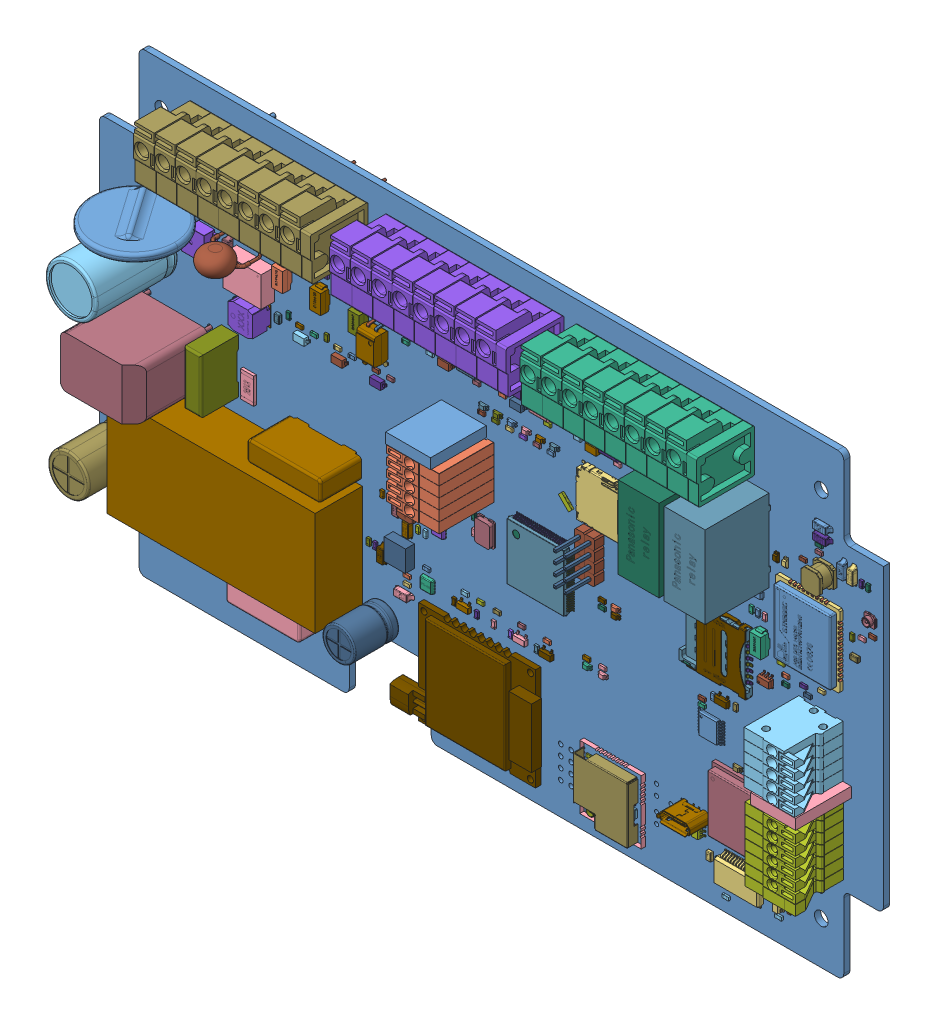
SolidWorks assembly Velvet_Controller_V1.2_2023, configuration Default. Lengths in mm. (continued)
Components (placement in the parent): (continued)
- Velvet_Controller_V1.2_2023(2)^Velvet_Controller_V1.2_2023-1: Velvet_Controller_V1.2_2023(2)^Velvet_Controller_V1.2_2023 [Default] at origin size (191.4 111.4 51.25) (virtual) (continued)
  - DD1gs^Velvet_Controller_V1.2_2023(2)_Velvet_Controller_V1.2_2023-1: DD1gs^Velvet_Controller_V1.2_2023(2)_Velvet_Controller_V1.2_2023 [Default] at origin size (15.7 17.6 2.34) (virtual) (continued)
    - SIM800C-1^DD1gs_Velvet_Controller_V1.2_2023(2)_Velvet_Controller_V1.2_2023-1: SIM800C-1^DD1gs_Velvet_Controller_V1.2_2023(2)_Velvet_Controller_V1.2_2023 [Default] at (173.7815 144.5582 -31.1) x (0 1 0) z (1 0 0) size (17.6 2.34 15.7) (virtual) (continued)
      - SIM800C_pads_D__faut^SIM800C-1_DD1gs_Velvet_Controller_V1.2_2023(2)_Velvet_Controller_V1.2_2023-15: SIM800C_pads_D__faut^SIM800C-1_DD1gs_Velvet_Controller_V1.2_2023(2)_Velvet_Controller_V1.2_2023 [Default] at (-66.1832 31.1435 -2.2565) x (0 0 -1) z (1 0 0) size (0.6 0.8 0.45) (virtual)
      - SIM800C_pads_D__faut^SIM800C-1_DD1gs_Velvet_Controller_V1.2_2023(2)_Velvet_Controller_V1.2_2023-16: SIM800C_pads_D__faut^SIM800C-1_DD1gs_Velvet_Controller_V1.2_2023(2)_Velvet_Controller_V1.2_2023 [Default] at (-66.1832 31.9435 -1.1565) x (0 0 1) z (1 0 0) size (0.6 0.8 0.45) (virtual)
      - SIM800C_pads_D__faut^SIM800C-1_DD1gs_Velvet_Controller_V1.2_2023(2)_Velvet_Controller_V1.2_2023-17: SIM800C_pads_D__faut^SIM800C-1_DD1gs_Velvet_Controller_V1.2_2023(2)_Velvet_Controller_V1.2_2023 [Default] at (-66.1832 31.9435 -0.0565) x (0 0 1) z (1 0 0) size (0.6 0.8 0.45) (virtual)
      - SIM800C_pads_D__faut^SIM800C-1_DD1gs_Velvet_Controller_V1.2_2023(2)_Velvet_Controller_V1.2_2023-18: SIM800C_pads_D__faut^SIM800C-1_DD1gs_Velvet_Controller_V1.2_2023(2)_Velvet_Controller_V1.2_2023 [Default] at (-66.1832 31.9435 1.0435) x (0 0 1) z (1 0 0) size (0.6 0.8 0.45) (virtual)
      - SIM800C_pads_D__faut^SIM800C-1_DD1gs_Velvet_Controller_V1.2_2023(2)_Velvet_Controller_V1.2_2023-19: SIM800C_pads_D__faut^SIM800C-1_DD1gs_Velvet_Controller_V1.2_2023(2)_Velvet_Controller_V1.2_2023 [Default] at (-66.1832 31.9435 2.1435) x (0 0 1) z (1 0 0) size (0.6 0.8 0.45) (virtual)
      - SIM800C_pads_D__faut^SIM800C-1_DD1gs_Velvet_Controller_V1.2_2023(2)_Velvet_Controller_V1.2_2023-20: SIM800C_pads_D__faut^SIM800C-1_DD1gs_Velvet_Controller_V1.2_2023(2)_Velvet_Controller_V1.2_2023 [Default] at (-66.1832 31.9435 3.2435) x (0 0 1) z (1 0 0) size (0.6 0.8 0.45) (virtual)
      - SIM800C_pads_D__faut^SIM800C-1_DD1gs_Velvet_Controller_V1.2_2023(2)_Velvet_Controller_V1.2_2023-21: SIM800C_pads_D__faut^SIM800C-1_DD1gs_Velvet_Controller_V1.2_2023(2)_Velvet_Controller_V1.2_2023 [Default] at (-66.1832 31.9435 4.3435) x (0 0 1) z (1 0 0) size (0.6 0.8 0.45) (virtual)
      - SIM800C_pads_D__faut^SIM800C-1_DD1gs_Velvet_Controller_V1.2_2023(2)_Velvet_Controller_V1.2_2023-22: SIM800C_pads_D__faut^SIM800C-1_DD1gs_Velvet_Controller_V1.2_2023(2)_Velvet_Controller_V1.2_2023 [Default] at (-83.3332 31.9435 -4.4565) x (0 0 -1) z (-1 0 0) size (0.6 0.8 0.45) (virtual)
      - SIM800C_pads_D__faut^SIM800C-1_DD1gs_Velvet_Controller_V1.2_2023(2)_Velvet_Controller_V1.2_2023-23: SIM800C_pads_D__faut^SIM800C-1_DD1gs_Velvet_Controller_V1.2_2023(2)_Velvet_Controller_V1.2_2023 [Default] at (-83.3332 31.1435 -3.3565) x (0 0 1) z (-1 0 0) size (0.6 0.8 0.45) (virtual)
      - SIM800C_pads_D__faut^SIM800C-1_DD1gs_Velvet_Controller_V1.2_2023(2)_Velvet_Controller_V1.2_2023-24: SIM800C_pads_D__faut^SIM800C-1_DD1gs_Velvet_Controller_V1.2_2023(2)_Velvet_Controller_V1.2_2023 [Default] at (-83.3332 31.1435 -2.2565) x (0 0 1) z (-1 0 0) size (0.6 0.8 0.45) (virtual)
      - SIM800C_pads_D__faut^SIM800C-1_DD1gs_Velvet_Controller_V1.2_2023(2)_Velvet_Controller_V1.2_2023-25: SIM800C_pads_D__faut^SIM800C-1_DD1gs_Velvet_Controller_V1.2_2023(2)_Velvet_Controller_V1.2_2023 [Default] at (-83.3332 31.1435 -1.1565) x (0 0 1) z (-1 0 0) size (0.6 0.8 0.45) (virtual)
      - SIM800C_pads_D__faut^SIM800C-1_DD1gs_Velvet_Controller_V1.2_2023(2)_Velvet_Controller_V1.2_2023-26: SIM800C_pads_D__faut^SIM800C-1_DD1gs_Velvet_Controller_V1.2_2023(2)_Velvet_Controller_V1.2_2023 [Default] at (-83.3332 31.1435 -0.0565) x (0 0 1) z (-1 0 0) size (0.6 0.8 0.45) (virtual)
      - SIM800C_pads_D__faut^SIM800C-1_DD1gs_Velvet_Controller_V1.2_2023(2)_Velvet_Controller_V1.2_2023-27: SIM800C_pads_D__faut^SIM800C-1_DD1gs_Velvet_Controller_V1.2_2023(2)_Velvet_Controller_V1.2_2023 [Default] at (-83.3332 31.1435 1.0435) x (0 0 1) z (-1 0 0) size (0.6 0.8 0.45) (virtual)
      - SIM800C_pads_D__faut^SIM800C-1_DD1gs_Velvet_Controller_V1.2_2023(2)_Velvet_Controller_V1.2_2023-28: SIM800C_pads_D__faut^SIM800C-1_DD1gs_Velvet_Controller_V1.2_2023(2)_Velvet_Controller_V1.2_2023 [Default] at (-83.3332 31.1435 2.1435) x (0 0 1) z (-1 0 0) size (0.6 0.8 0.45) (virtual)
      - SIM800C_pads_D__faut^SIM800C-1_DD1gs_Velvet_Controller_V1.2_2023(2)_Velvet_Controller_V1.2_2023-29: SIM800C_pads_D__faut^SIM800C-1_DD1gs_Velvet_Controller_V1.2_2023(2)_Velvet_Controller_V1.2_2023 [Default] at (-83.3332 31.1435 3.2435) x (0 0 1) z (-1 0 0) size (0.6 0.8 0.45) (virtual)
      - SIM800C_pads_D__faut^SIM800C-1_DD1gs_Velvet_Controller_V1.2_2023(2)_Velvet_Controller_V1.2_2023-30: SIM800C_pads_D__faut^SIM800C-1_DD1gs_Velvet_Controller_V1.2_2023(2)_Velvet_Controller_V1.2_2023 [Default] at (-83.3332 31.1435 4.3435) x (0 0 1) z (-1 0 0) size (0.6 0.8 0.45) (virtual)
      - SIM800C_pads_D__faut^SIM800C-1_DD1gs_Velvet_Controller_V1.2_2023(2)_Velvet_Controller_V1.2_2023-31: SIM800C_pads_D__faut^SIM800C-1_DD1gs_Velvet_Controller_V1.2_2023(2)_Velvet_Controller_V1.2_2023 [Default] at (-80.8082 31.9435 7.5685) x (-1 0 0) z (0 0 1) size (0.6 0.8 0.45) (virtual)
      - SIM800C_pads_D__faut^SIM800C-1_DD1gs_Velvet_Controller_V1.2_2023(2)_Velvet_Controller_V1.2_2023-32: SIM800C_pads_D__faut^SIM800C-1_DD1gs_Velvet_Controller_V1.2_2023(2)_Velvet_Controller_V1.2_2023 [Default] at (-79.7082 31.1435 7.5685) size (0.6 0.8 0.45) (virtual)
      - SIM800C_pads_D__faut^SIM800C-1_DD1gs_Velvet_Controller_V1.2_2023(2)_Velvet_Controller_V1.2_2023-33: SIM800C_pads_D__faut^SIM800C-1_DD1gs_Velvet_Controller_V1.2_2023(2)_Velvet_Controller_V1.2_2023 [Default] at (-78.6082 31.9435 7.5685) x (-1 0 0) z (0 0 1) size (0.6 0.8 0.45) (virtual)
      - SIM800C_pads_D__faut^SIM800C-1_DD1gs_Velvet_Controller_V1.2_2023(2)_Velvet_Controller_V1.2_2023-34: SIM800C_pads_D__faut^SIM800C-1_DD1gs_Velvet_Controller_V1.2_2023(2)_Velvet_Controller_V1.2_2023 [Default] at (-77.5082 31.9435 7.5685) x (-1 0 0) z (0 0 1) size (0.6 0.8 0.45) (virtual)
      - SIM800C_pads_D__faut^SIM800C-1_DD1gs_Velvet_Controller_V1.2_2023(2)_Velvet_Controller_V1.2_2023-35: SIM800C_pads_D__faut^SIM800C-1_DD1gs_Velvet_Controller_V1.2_2023(2)_Velvet_Controller_V1.2_2023 [Default] at (-76.4082 31.1435 7.5685) size (0.6 0.8 0.45) (virtual)
      - SIM800C_pads_D__faut^SIM800C-1_DD1gs_Velvet_Controller_V1.2_2023(2)_Velvet_Controller_V1.2_2023-36: SIM800C_pads_D__faut^SIM800C-1_DD1gs_Velvet_Controller_V1.2_2023(2)_Velvet_Controller_V1.2_2023 [Default] at (-75.3082 31.1435 7.5685) size (0.6 0.8 0.45) (virtual)
      - SIM800C_pads_D__faut^SIM800C-1_DD1gs_Velvet_Controller_V1.2_2023(2)_Velvet_Controller_V1.2_2023-37: SIM800C_pads_D__faut^SIM800C-1_DD1gs_Velvet_Controller_V1.2_2023(2)_Velvet_Controller_V1.2_2023 [Default] at (-74.2082 31.1435 7.5685) size (0.6 0.8 0.45) (virtual)
      - SIM800C_pads_D__faut^SIM800C-1_DD1gs_Velvet_Controller_V1.2_2023(2)_Velvet_Controller_V1.2_2023-38: SIM800C_pads_D__faut^SIM800C-1_DD1gs_Velvet_Controller_V1.2_2023(2)_Velvet_Controller_V1.2_2023 [Default] at (-73.1082 31.1435 7.5685) size (0.6 0.8 0.45) (virtual)
      - SIM800C_pads_D__faut^SIM800C-1_DD1gs_Velvet_Controller_V1.2_2023(2)_Velvet_Controller_V1.2_2023-39: SIM800C_pads_D__faut^SIM800C-1_DD1gs_Velvet_Controller_V1.2_2023(2)_Velvet_Controller_V1.2_2023 [Default] at (-72.0082 31.1435 7.5685) size (0.6 0.8 0.45) (virtual)
      - SIM800C_pads_D__faut^SIM800C-1_DD1gs_Velvet_Controller_V1.2_2023(2)_Velvet_Controller_V1.2_2023-40: SIM800C_pads_D__faut^SIM800C-1_DD1gs_Velvet_Controller_V1.2_2023(2)_Velvet_Controller_V1.2_2023 [Default] at (-70.9082 31.1435 7.5685) size (0.6 0.8 0.45) (virtual)
      - SIM800C_pads_D__faut^SIM800C-1_DD1gs_Velvet_Controller_V1.2_2023(2)_Velvet_Controller_V1.2_2023-41: SIM800C_pads_D__faut^SIM800C-1_DD1gs_Velvet_Controller_V1.2_2023(2)_Velvet_Controller_V1.2_2023 [Default] at (-69.8082 31.1435 7.5685) size (0.6 0.8 0.45) (virtual)
      - SIM800C_pads_D__faut^SIM800C-1_DD1gs_Velvet_Controller_V1.2_2023(2)_Velvet_Controller_V1.2_2023-42: SIM800C_pads_D__faut^SIM800C-1_DD1gs_Velvet_Controller_V1.2_2023(2)_Velvet_Controller_V1.2_2023 [Default] at (-68.7082 31.1435 7.5685) size (0.6 0.8 0.45) (virtual)
  - DA5p^Velvet_Controller_V1.2_2023(2)_Velvet_Controller_V1.2_2023-1: DA5p^Velvet_Controller_V1.2_2023(2)_Velvet_Controller_V1.2_2023 [Default] at origin size (9.3 7.32 3.41) (virtual)
    - B05xxMT-1WR4_MNS^DA5p_Velvet_Controller_V1.2_2023(2)_Velvet_Controller_V1.2_2023-1: B05xxMT-1WR4_MNS^DA5p_Velvet_Controller_V1.2_2023(2)_Velvet_Controller_V1.2_2023 [Default] at (38.2 77.8 0) x (0 -1 0) z (0 0 1) size (7.32 9.3 3.41) (virtual)
  - DA4p^Velvet_Controller_V1.2_2023(2)_Velvet_Controller_V1.2_2023-1: DA4p^Velvet_Controller_V1.2_2023(2)_Velvet_Controller_V1.2_2023 [Default] at origin size (3.2 3.1 0.81) (virtual)
    - DFN_3x3_8L_EP2_P^DA4p_Velvet_Controller_V1.2_2023(2)_Velvet_Controller_V1.2_2023-1: DFN_3x3_8L_EP2_P^DA4p_Velvet_Controller_V1.2_2023(2)_Velvet_Controller_V1.2_2023 [Default] at (80.4 33.275 0) x (0 -1 0) z (-1 0 0) size (3.1 0.81 3.2) (virtual)
      - lead frame^DFN_3x3_8L_EP2_P_DA4p_Velvet_Controller_V1.2_2023(2)_Velvet_Controller_V1.2_2023-1: lead frame^DFN_3x3_8L_EP2_P_DA4p_Velvet_Controller_V1.2_2023(2)_Velvet_Controller_V1.2_2023 [Default] x (0 0 1) z (0 1 0) size (3.2 3.1 0.15) (virtual)
      - Body^DFN_3x3_8L_EP2_P_DA4p_Velvet_Controller_V1.2_2023(2)_Velvet_Controller_V1.2_2023-1: Body^DFN_3x3_8L_EP2_P_DA4p_Velvet_Controller_V1.2_2023(2)_Velvet_Controller_V1.2_2023 [Default] at (0 0.01 0) x (0 0 -1) z (1 0 0) size (3 0.8 3) (virtual)
  - DA3p^Velvet_Controller_V1.2_2023(2)_Velvet_Controller_V1.2_2023-1: DA3p^Velvet_Controller_V1.2_2023(2)_Velvet_Controller_V1.2_2023 [Default] at origin size (3.2 3.1 0.81) (virtual)
    - DFN_3x3_8L_EP2_P^DA3p_Velvet_Controller_V1.2_2023(2)_Velvet_Controller_V1.2_2023-1: DFN_3x3_8L_EP2_P^DA3p_Velvet_Controller_V1.2_2023(2)_Velvet_Controller_V1.2_2023 [Default] at (83.1247 46.2693 0) x (0 -1 0) z (-1 0 0) size (3.1 0.81 3.2) (virtual)
      - lead frame^DFN_3x3_8L_EP2_P_DA3p_Velvet_Controller_V1.2_2023(2)_Velvet_Controller_V1.2_2023-1: lead frame^DFN_3x3_8L_EP2_P_DA3p_Velvet_Controller_V1.2_2023(2)_Velvet_Controller_V1.2_2023 [Default] x (0 0 1) z (0 1 0) size (3.2 3.1 0.15) (virtual)
      - Body^DFN_3x3_8L_EP2_P_DA3p_Velvet_Controller_V1.2_2023(2)_Velvet_Controller_V1.2_2023-1: Body^DFN_3x3_8L_EP2_P_DA3p_Velvet_Controller_V1.2_2023(2)_Velvet_Controller_V1.2_2023 [Default] at (0 0.01 0) x (0 0 -1) z (1 0 0) size (3 0.8 3) (virtual)
  - DA2p^Velvet_Controller_V1.2_2023(2)_Velvet_Controller_V1.2_2023-1: DA2p^Velvet_Controller_V1.2_2023(2)_Velvet_Controller_V1.2_2023 [Default] at origin (virtual)
    - DFN_3x3_8L_EP2_P.step-1: DFN_3x3_8L_EP2_P.step [Default] at (172.1 87.075 0) x (0 1 0) z (1 0 0) (suppressed, hidden)
  - DA1p^Velvet_Controller_V1.2_2023(2)_Velvet_Controller_V1.2_2023-1: DA1p^Velvet_Controller_V1.2_2023(2)_Velvet_Controller_V1.2_2023 [Default] at origin size (50.8 25.4 11.55) (virtual)
    - 6302613216^DA1p_Velvet_Controller_V1.2_2023(2)_Velvet_Controller_V1.2_2023-1: 6302613216^DA1p_Velvet_Controller_V1.2_2023(2)_Velvet_Controller_V1.2_2023 [Default] at (39.06 33.34 0.254) size (50.8 25.4 11.55) (virtual)
      - Extruded-6^6302613216_DA1p_Velvet_Controller_V1.2_2023(2)_Velvet_Controller_V1.2_2023-1: Extruded-6^6302613216_DA1p_Velvet_Controller_V1.2_2023(2)_Velvet_Controller_V1.2_2023 [Default] at origin size (50.8 25.4 11.55) (virtual)
  - C41p^Velvet_Controller_V1.2_2023(2)_Velvet_Controller_V1.2_2023-1: C41p^Velvet_Controller_V1.2_2023(2)_Velvet_Controller_V1.2_2023 [Default] at origin size (0.8 1.6 0.5) (virtual)
    - CAP 0603 (1608)^C41p_Velvet_Controller_V1.2_2023(2)_Velvet_Controller_V1.2_2023-1: CAP 0603 (1608)^C41p_Velvet_Controller_V1.2_2023(2)_Velvet_Controller_V1.2_2023 [Default] at (82.775 30.3 -1.5) x (0 -1 0) z (1 0 0) size (1.6 0.5 0.8) (virtual)
  - C40p^Velvet_Controller_V1.2_2023(2)_Velvet_Controller_V1.2_2023-1: C40p^Velvet_Controller_V1.2_2023(2)_Velvet_Controller_V1.2_2023 [Default] at origin size (9.03 5 42.27) (virtual)
    - VY2100K29U2JS63V7^C40p_Velvet_Controller_V1.2_2023(2)_Velvet_Controller_V1.2_2023-1: VY2100K29U2JS63V7^C40p_Velvet_Controller_V1.2_2023(2)_Velvet_Controller_V1.2_2023 [Default] at (38.3 86.075 10) x (-1 0 0) z (0 0 1) size (9.03 5 42.27) (virtual)
  - C39p^Velvet_Controller_V1.2_2023(2)_Velvet_Controller_V1.2_2023-1: C39p^Velvet_Controller_V1.2_2023(2)_Velvet_Controller_V1.2_2023 [Default] at origin size (0.8 1.6 0.5) (virtual)
    - CAP 0603 (1608)^C39p_Velvet_Controller_V1.2_2023(2)_Velvet_Controller_V1.2_2023-1: CAP 0603 (1608)^C39p_Velvet_Controller_V1.2_2023(2)_Velvet_Controller_V1.2_2023 [Default] at (80.95 30.3 -1.5) x (0 -1 0) z (1 0 0) size (1.6 0.5 0.8) (virtual)
  - C38p^Velvet_Controller_V1.2_2023(2)_Velvet_Controller_V1.2_2023-1: C38p^Velvet_Controller_V1.2_2023(2)_Velvet_Controller_V1.2_2023 [Default] at origin size (1.62 4.56 1.51) (virtual)
    - CAP 1206^C38p_Velvet_Controller_V1.2_2023(2)_Velvet_Controller_V1.2_2023-1: CAP 1206^C38p_Velvet_Controller_V1.2_2023(2)_Velvet_Controller_V1.2_2023 [Default] at (31.9 80.55 0) x (0 -1 0) z (0 0 1) size (4.56 1.62 1.51) (virtual)
  - C37p^Velvet_Controller_V1.2_2023(2)_Velvet_Controller_V1.2_2023-1: C37p^Velvet_Controller_V1.2_2023(2)_Velvet_Controller_V1.2_2023 [Default] at origin size (1.25 2 0.78) (virtual)
    - CAP 0805^C37p_Velvet_Controller_V1.2_2023(2)_Velvet_Controller_V1.2_2023-1: CAP 0805^C37p_Velvet_Controller_V1.2_2023(2)_Velvet_Controller_V1.2_2023 [Default] at (44 71.4 0) x (0 -1 0) z (-1 0 0) size (2 0.78 1.25) (virtual)
  - C36p^Velvet_Controller_V1.2_2023(2)_Velvet_Controller_V1.2_2023-1: C36p^Velvet_Controller_V1.2_2023(2)_Velvet_Controller_V1.2_2023 [Default] at origin size (1.25 2 0.78) (virtual)
    - CAP 0805^C36p_Velvet_Controller_V1.2_2023(2)_Velvet_Controller_V1.2_2023-1: CAP 0805^C36p_Velvet_Controller_V1.2_2023(2)_Velvet_Controller_V1.2_2023 [Default] at (33.8 69.6 0) x (0 1 0) z (1 0 0) size (2 0.78 1.25) (virtual)
  - C35p^Velvet_Controller_V1.2_2023(2)_Velvet_Controller_V1.2_2023-1: C35p^Velvet_Controller_V1.2_2023(2)_Velvet_Controller_V1.2_2023 [Default] at origin size (0.8 1.6 0.5) (virtual)
    - CAP 0603 (1608)^C35p_Velvet_Controller_V1.2_2023(2)_Velvet_Controller_V1.2_2023-1: CAP 0603 (1608)^C35p_Velvet_Controller_V1.2_2023(2)_Velvet_Controller_V1.2_2023 [Default] at (65.6 35.9 0) x (0 -1 0) z (-1 0 0) size (1.6 0.5 0.8) (virtual)
  - C34p^Velvet_Controller_V1.2_2023(2)_Velvet_Controller_V1.2_2023-1: C34p^Velvet_Controller_V1.2_2023(2)_Velvet_Controller_V1.2_2023 [Default] at origin size (0.8 1.6 0.5) (virtual)
    - CAP 0603 (1608)^C34p_Velvet_Controller_V1.2_2023(2)_Velvet_Controller_V1.2_2023-1: CAP 0603 (1608)^C34p_Velvet_Controller_V1.2_2023(2)_Velvet_Controller_V1.2_2023 [Default] at (67.2 35.9 0) x (0 -1 0) z (-1 0 0) size (1.6 0.5 0.8) (virtual)
  - C33p^Velvet_Controller_V1.2_2023(2)_Velvet_Controller_V1.2_2023-1: C33p^Velvet_Controller_V1.2_2023(2)_Velvet_Controller_V1.2_2023 [Default] at origin size (1.62 4.56 1.51) (virtual)
    - CAP 1206^C33p_Velvet_Controller_V1.2_2023(2)_Velvet_Controller_V1.2_2023-1: CAP 1206^C33p_Velvet_Controller_V1.2_2023(2)_Velvet_Controller_V1.2_2023 [Default] at (69.6 34.3 0) x (0 1 0) z (0 0 1) size (4.56 1.62 1.51) (virtual)
  - C32p^Velvet_Controller_V1.2_2023(2)_Velvet_Controller_V1.2_2023-1: C32p^Velvet_Controller_V1.2_2023(2)_Velvet_Controller_V1.2_2023 [Default] at origin size (1.6 0.8 0.5) (virtual)
    - CAP 0603 (1608)^C32p_Velvet_Controller_V1.2_2023(2)_Velvet_Controller_V1.2_2023-1: CAP 0603 (1608)^C32p_Velvet_Controller_V1.2_2023(2)_Velvet_Controller_V1.2_2023 [Default] at (81 36.85 0) x (-1 0 0) z (0 1 0) size (1.6 0.5 0.8) (virtual)
  - C31p^Velvet_Controller_V1.2_2023(2)_Velvet_Controller_V1.2_2023-1: C31p^Velvet_Controller_V1.2_2023(2)_Velvet_Controller_V1.2_2023 [Default] at origin size (1.6 0.8 0.5) (virtual)
    - CAP 0603 (1608)^C31p_Velvet_Controller_V1.2_2023(2)_Velvet_Controller_V1.2_2023-1: CAP 0603 (1608)^C31p_Velvet_Controller_V1.2_2023(2)_Velvet_Controller_V1.2_2023 [Default] at (76.2 32.95 0) x (-1 0 0) z (0 1 0) size (1.6 0.5 0.8) (virtual)
  - C30p^Velvet_Controller_V1.2_2023(2)_Velvet_Controller_V1.2_2023-1: C30p^Velvet_Controller_V1.2_2023(2)_Velvet_Controller_V1.2_2023 [Default] at origin size (1.6 0.8 0.5) (virtual)
    - CAP 0603 (1608)^C30p_Velvet_Controller_V1.2_2023(2)_Velvet_Controller_V1.2_2023-1: CAP 0603 (1608)^C30p_Velvet_Controller_V1.2_2023(2)_Velvet_Controller_V1.2_2023 [Default] at (76.2 31.15 0) x (-1 0 0) z (0 1 0) size (1.6 0.5 0.8) (virtual)
  - C29p^Velvet_Controller_V1.2_2023(2)_Velvet_Controller_V1.2_2023-1: C29p^Velvet_Controller_V1.2_2023(2)_Velvet_Controller_V1.2_2023 [Default] at origin size (4.56 1.62 1.51) (virtual)
    - CAP 1206^C29p_Velvet_Controller_V1.2_2023(2)_Velvet_Controller_V1.2_2023-1: CAP 1206^C29p_Velvet_Controller_V1.2_2023(2)_Velvet_Controller_V1.2_2023 [Default] at (74.6 28.45 0) x (1 0 0) z (0 0 1) size (4.56 1.62 1.51) (virtual)
  - C28p^Velvet_Controller_V1.2_2023(2)_Velvet_Controller_V1.2_2023-1: C28p^Velvet_Controller_V1.2_2023(2)_Velvet_Controller_V1.2_2023 [Default] at origin size (0.8 1.6 0.5) (virtual)
    - CAP 0603 (1608)^C28p_Velvet_Controller_V1.2_2023(2)_Velvet_Controller_V1.2_2023-1: CAP 0603 (1608)^C28p_Velvet_Controller_V1.2_2023(2)_Velvet_Controller_V1.2_2023 [Default] at (85.4247 42.6693 -1.5) x (0 -1 0) z (1 0 0) size (1.6 0.5 0.8) (virtual)
  - C27p^Velvet_Controller_V1.2_2023(2)_Velvet_Controller_V1.2_2023-1: C27p^Velvet_Controller_V1.2_2023(2)_Velvet_Controller_V1.2_2023 [Default] at origin size (0.8 1.6 0.5) (virtual)
    - CAP 0603 (1608)^C27p_Velvet_Controller_V1.2_2023(2)_Velvet_Controller_V1.2_2023-1: CAP 0603 (1608)^C27p_Velvet_Controller_V1.2_2023(2)_Velvet_Controller_V1.2_2023 [Default] at (169.6 90.2 -1.5) x (0 1 0) z (-1 0 0) size (1.6 0.5 0.8) (virtual)
  - C26p^Velvet_Controller_V1.2_2023(2)_Velvet_Controller_V1.2_2023-1: C26p^Velvet_Controller_V1.2_2023(2)_Velvet_Controller_V1.2_2023 [Default] at origin size (0.8 1.6 0.5) (virtual)
    - CAP 0603 (1608)^C26p_Velvet_Controller_V1.2_2023(2)_Velvet_Controller_V1.2_2023-1: CAP 0603 (1608)^C26p_Velvet_Controller_V1.2_2023(2)_Velvet_Controller_V1.2_2023 [Default] at (171.3 90.2 -1.5) x (0 1 0) z (-1 0 0) size (1.6 0.5 0.8) (virtual)
  - C25p^Velvet_Controller_V1.2_2023(2)_Velvet_Controller_V1.2_2023-1: C25p^Velvet_Controller_V1.2_2023(2)_Velvet_Controller_V1.2_2023 [Default] at origin size (0.8 1.6 0.5) (virtual)
    - CAP 0603 (1608)^C25p_Velvet_Controller_V1.2_2023(2)_Velvet_Controller_V1.2_2023-1: CAP 0603 (1608)^C25p_Velvet_Controller_V1.2_2023(2)_Velvet_Controller_V1.2_2023 [Default] at (83.6247 42.6693 -1.5) x (0 -1 0) z (1 0 0) size (1.6 0.5 0.8) (virtual)
  - C24p^Velvet_Controller_V1.2_2023(2)_Velvet_Controller_V1.2_2023-1: C24p^Velvet_Controller_V1.2_2023(2)_Velvet_Controller_V1.2_2023 [Default] at origin size (0.8 1.6 0.5) (virtual)
    - CAP 0603 (1608)^C24p_Velvet_Controller_V1.2_2023(2)_Velvet_Controller_V1.2_2023-1: CAP 0603 (1608)^C24p_Velvet_Controller_V1.2_2023(2)_Velvet_Controller_V1.2_2023 [Default] at (68.9247 47.6693 0) x (0 -1 0) z (-1 0 0) size (1.6 0.5 0.8) (virtual)
  - C24mc^Velvet_Controller_V1.2_2023(2)_Velvet_Controller_V1.2_2023-1: C24mc^Velvet_Controller_V1.2_2023(2)_Velvet_Controller_V1.2_2023 [Default] at origin size (0.8 1.6 0.5) (virtual)
    - CAP 0603 (1608)^C24mc_Velvet_Controller_V1.2_2023(2)_Velvet_Controller_V1.2_2023-1: CAP 0603 (1608)^C24mc_Velvet_Controller_V1.2_2023(2)_Velvet_Controller_V1.2_2023 [Default] at (126.225 72.55 -1.5) x (0 -1 0) z (1 0 0) size (1.6 0.5 0.8) (virtual)
  - C23p^Velvet_Controller_V1.2_2023(2)_Velvet_Controller_V1.2_2023-1: C23p^Velvet_Controller_V1.2_2023(2)_Velvet_Controller_V1.2_2023 [Default] at origin size (0.8 1.6 0.5) (virtual)
    - CAP 0603 (1608)^C23p_Velvet_Controller_V1.2_2023(2)_Velvet_Controller_V1.2_2023-1: CAP 0603 (1608)^C23p_Velvet_Controller_V1.2_2023(2)_Velvet_Controller_V1.2_2023 [Default] at (70.7247 47.6693 0) x (0 -1 0) z (-1 0 0) size (1.6 0.5 0.8) (virtual)
  - C23mc^Velvet_Controller_V1.2_2023(2)_Velvet_Controller_V1.2_2023-1: C23mc^Velvet_Controller_V1.2_2023(2)_Velvet_Controller_V1.2_2023 [Default] at origin size (0.8 1.6 0.5) (virtual)
    - CAP 0603 (1608)^C23mc_Velvet_Controller_V1.2_2023(2)_Velvet_Controller_V1.2_2023-1: CAP 0603 (1608)^C23mc_Velvet_Controller_V1.2_2023(2)_Velvet_Controller_V1.2_2023 [Default] at (126.875 70.975 -1.5) x (0 1 0) z (-1 0 0) size (1.6 0.5 0.8) (virtual)
  - C22p^Velvet_Controller_V1.2_2023(2)_Velvet_Controller_V1.2_2023-1: C22p^Velvet_Controller_V1.2_2023(2)_Velvet_Controller_V1.2_2023 [Default] at origin size (1.62 4.56 1.51) (virtual)
    - CAP 1206^C22p_Velvet_Controller_V1.2_2023(2)_Velvet_Controller_V1.2_2023-1: CAP 1206^C22p_Velvet_Controller_V1.2_2023(2)_Velvet_Controller_V1.2_2023 [Default] at (73.3248 46.0693 0) x (0 1 0) z (0 0 1) size (4.56 1.62 1.51) (virtual)
  - C22mc^Velvet_Controller_V1.2_2023(2)_Velvet_Controller_V1.2_2023-1: C22mc^Velvet_Controller_V1.2_2023(2)_Velvet_Controller_V1.2_2023 [Default] at origin size (1.25 2 0.78) (virtual)
    - CAP 0805^C22mc_Velvet_Controller_V1.2_2023(2)_Velvet_Controller_V1.2_2023-1: CAP 0805^C22mc_Velvet_Controller_V1.2_2023(2)_Velvet_Controller_V1.2_2023 [Default] at (102.325 55.95 -1.5) x (0 -1 0) z (1 0 0) size (2 0.78 1.25) (virtual)
  - C21p^Velvet_Controller_V1.2_2023(2)_Velvet_Controller_V1.2_2023-1: C21p^Velvet_Controller_V1.2_2023(2)_Velvet_Controller_V1.2_2023 [Default] at origin size (0.8 1.6 0.5) (virtual)
    - CAP 0603 (1608)^C21p_Velvet_Controller_V1.2_2023(2)_Velvet_Controller_V1.2_2023-1: CAP 0603 (1608)^C21p_Velvet_Controller_V1.2_2023(2)_Velvet_Controller_V1.2_2023 [Default] at (188.3 85.5 0) x (0 1 0) z (1 0 0) size (1.6 0.5 0.8) (virtual)
  - C21mc^Velvet_Controller_V1.2_2023(2)_Velvet_Controller_V1.2_2023-1: C21mc^Velvet_Controller_V1.2_2023(2)_Velvet_Controller_V1.2_2023 [Default] at origin size (0.8 1.6 0.5) (virtual)
    - CAP 0603 (1608)^C21mc_Velvet_Controller_V1.2_2023(2)_Velvet_Controller_V1.2_2023-1: CAP 0603 (1608)^C21mc_Velvet_Controller_V1.2_2023(2)_Velvet_Controller_V1.2_2023 [Default] at (101.025 56.925 -1.5) x (0 -1 0) z (1 0 0) size (1.6 0.5 0.8) (virtual)
  - C20p^Velvet_Controller_V1.2_2023(2)_Velvet_Controller_V1.2_2023-1: C20p^Velvet_Controller_V1.2_2023(2)_Velvet_Controller_V1.2_2023 [Default] at origin size (0.8 1.6 0.5) (virtual)
    - CAP 0603 (1608)^C20p_Velvet_Controller_V1.2_2023(2)_Velvet_Controller_V1.2_2023-1: CAP 0603 (1608)^C20p_Velvet_Controller_V1.2_2023(2)_Velvet_Controller_V1.2_2023 [Default] at (186.7 85.5 0) x (0 1 0) z (1 0 0) size (1.6 0.5 0.8) (virtual)
  - C20mc^Velvet_Controller_V1.2_2023(2)_Velvet_Controller_V1.2_2023-1: C20mc^Velvet_Controller_V1.2_2023(2)_Velvet_Controller_V1.2_2023 [Default] at origin size (1.6 0.8 0.5) (virtual)
    - CAP 0603 (1608)^C20mc_Velvet_Controller_V1.2_2023(2)_Velvet_Controller_V1.2_2023-1: CAP 0603 (1608)^C20mc_Velvet_Controller_V1.2_2023(2)_Velvet_Controller_V1.2_2023 [Default] at (115.725 59.15 -1.5) x (-1 0 0) z (0 -1 0) size (1.6 0.5 0.8) (virtual)
  - C19p^Velvet_Controller_V1.2_2023(2)_Velvet_Controller_V1.2_2023-1: C19p^Velvet_Controller_V1.2_2023(2)_Velvet_Controller_V1.2_2023 [Default] at origin size (1.62 4.56 1.51) (virtual)
    - CAP 1206^C19p_Velvet_Controller_V1.2_2023(2)_Velvet_Controller_V1.2_2023-1: CAP 1206^C19p_Velvet_Controller_V1.2_2023(2)_Velvet_Controller_V1.2_2023 [Default] at (181.9 87.1 0) x (0 -1 0) z (0 0 1) size (4.56 1.62 1.51) (virtual)
  - C19mc^Velvet_Controller_V1.2_2023(2)_Velvet_Controller_V1.2_2023-1: C19mc^Velvet_Controller_V1.2_2023(2)_Velvet_Controller_V1.2_2023 [Default] at origin size (1.6 0.8 0.5) (virtual)
    - CAP 0603 (1608)^C19mc_Velvet_Controller_V1.2_2023(2)_Velvet_Controller_V1.2_2023-1: CAP 0603 (1608)^C19mc_Velvet_Controller_V1.2_2023(2)_Velvet_Controller_V1.2_2023 [Default] at (100.7 53.425 -1.5) x (1 0 0) z (0 1 0) size (1.6 0.5 0.8) (virtual)
  - C18p^Velvet_Controller_V1.2_2023(2)_Velvet_Controller_V1.2_2023-1: C18p^Velvet_Controller_V1.2_2023(2)_Velvet_Controller_V1.2_2023 [Default] at origin size (1.62 4.56 1.51) (virtual)
    - CAP 1206^C18p_Velvet_Controller_V1.2_2023(2)_Velvet_Controller_V1.2_2023-1: CAP 1206^C18p_Velvet_Controller_V1.2_2023(2)_Velvet_Controller_V1.2_2023 [Default] at (184.3 87.1 0) x (0 -1 0) z (0 0 1) size (4.56 1.62 1.51) (virtual)
  - C18mc^Velvet_Controller_V1.2_2023(2)_Velvet_Controller_V1.2_2023-1: C18mc^Velvet_Controller_V1.2_2023(2)_Velvet_Controller_V1.2_2023 [Default] at origin size (1.6 0.8 0.5) (virtual)
    - CAP 0603 (1608)^C18mc_Velvet_Controller_V1.2_2023(2)_Velvet_Controller_V1.2_2023-1: CAP 0603 (1608)^C18mc_Velvet_Controller_V1.2_2023(2)_Velvet_Controller_V1.2_2023 [Default] at (100.7 51.825 -1.5) x (1 0 0) z (0 1 0) size (1.6 0.5 0.8) (virtual)
  - C17p^Velvet_Controller_V1.2_2023(2)_Velvet_Controller_V1.2_2023-1: C17p^Velvet_Controller_V1.2_2023(2)_Velvet_Controller_V1.2_2023 [Default] at origin size (0.8 1.6 0.5) (virtual)
    - CAP 0603 (1608)^C17p_Velvet_Controller_V1.2_2023(2)_Velvet_Controller_V1.2_2023-1: CAP 0603 (1608)^C17p_Velvet_Controller_V1.2_2023(2)_Velvet_Controller_V1.2_2023 [Default] at (79.4247 44.4693 0) x (0 -1 0) z (-1 0 0) size (1.6 0.5 0.8) (virtual)
  - C17mc^Velvet_Controller_V1.2_2023(2)_Velvet_Controller_V1.2_2023-1: C17mc^Velvet_Controller_V1.2_2023(2)_Velvet_Controller_V1.2_2023 [Default] at origin size (0.8 1.6 0.5) (virtual)
    - CAP 0603 (1608)^C17mc_Velvet_Controller_V1.2_2023(2)_Velvet_Controller_V1.2_2023-1: CAP 0603 (1608)^C17mc_Velvet_Controller_V1.2_2023(2)_Velvet_Controller_V1.2_2023 [Default] at (103.575 45.175 -1.5) x (0 1 0) z (-1 0 0) size (1.6 0.5 0.8) (virtual)
  - C16p^Velvet_Controller_V1.2_2023(2)_Velvet_Controller_V1.2_2023-1: C16p^Velvet_Controller_V1.2_2023(2)_Velvet_Controller_V1.2_2023 [Default] at origin size (0.8 1.6 0.5) (virtual)
    - CAP 0603 (1608)^C16p_Velvet_Controller_V1.2_2023(2)_Velvet_Controller_V1.2_2023-1: CAP 0603 (1608)^C16p_Velvet_Controller_V1.2_2023(2)_Velvet_Controller_V1.2_2023 [Default] at (77.6247 44.4693 0) x (0 -1 0) z (-1 0 0) size (1.6 0.5 0.8) (virtual)
  - C16mc^Velvet_Controller_V1.2_2023(2)_Velvet_Controller_V1.2_2023-1: C16mc^Velvet_Controller_V1.2_2023(2)_Velvet_Controller_V1.2_2023 [Default] at origin size (1.6 0.8 0.5) (virtual)
    - CAP 0603 (1608)^C16mc_Velvet_Controller_V1.2_2023(2)_Velvet_Controller_V1.2_2023-1: CAP 0603 (1608)^C16mc_Velvet_Controller_V1.2_2023(2)_Velvet_Controller_V1.2_2023 [Default] at (115.725 57.55 -1.5) x (-1 0 0) z (0 -1 0) size (1.6 0.5 0.8) (virtual)
  - C15p^Velvet_Controller_V1.2_2023(2)_Velvet_Controller_V1.2_2023-1: C15p^Velvet_Controller_V1.2_2023(2)_Velvet_Controller_V1.2_2023 [Default] at origin size (1.62 4.56 1.51) (virtual)
    - CAP 1206^C15p_Velvet_Controller_V1.2_2023(2)_Velvet_Controller_V1.2_2023-1: CAP 1206^C15p_Velvet_Controller_V1.2_2023(2)_Velvet_Controller_V1.2_2023 [Default] at (75.8 42.9 0) x (0 1 0) z (0 0 1) size (4.56 1.62 1.51) (virtual)
  - C15mc^Velvet_Controller_V1.2_2023(2)_Velvet_Controller_V1.2_2023-1: C15mc^Velvet_Controller_V1.2_2023(2)_Velvet_Controller_V1.2_2023 [Default] at origin size (0.8 1.6 0.5) (virtual)
    - CAP 0603 (1608)^C15mc_Velvet_Controller_V1.2_2023(2)_Velvet_Controller_V1.2_2023-1: CAP 0603 (1608)^C15mc_Velvet_Controller_V1.2_2023(2)_Velvet_Controller_V1.2_2023 [Default] at (104.375 56.925 -1.5) x (0 -1 0) z (1 0 0) size (1.6 0.5 0.8) (virtual)
  - C14p^Velvet_Controller_V1.2_2023(2)_Velvet_Controller_V1.2_2023-1: C14p^Velvet_Controller_V1.2_2023(2)_Velvet_Controller_V1.2_2023 [Default] at origin size (1.6 0.8 0.5) (virtual)
    - CAP 0603 (1608)^C14p_Velvet_Controller_V1.2_2023(2)_Velvet_Controller_V1.2_2023-1: CAP 0603 (1608)^C14p_Velvet_Controller_V1.2_2023(2)_Velvet_Controller_V1.2_2023 [Default] at (171.3 84 0) x (1 0 0) z (0 -1 0) size (1.6 0.5 0.8) (virtual)
  - C14mc^Velvet_Controller_V1.2_2023(2)_Velvet_Controller_V1.2_2023-1: C14mc^Velvet_Controller_V1.2_2023(2)_Velvet_Controller_V1.2_2023 [Default] at origin size (1.6 0.8 0.5) (virtual)
    - CAP 0603 (1608)^C14mc_Velvet_Controller_V1.2_2023(2)_Velvet_Controller_V1.2_2023-1: CAP 0603 (1608)^C14mc_Velvet_Controller_V1.2_2023(2)_Velvet_Controller_V1.2_2023 [Default] at (100.7 50.25 -1.5) x (1 0 0) z (0 1 0) size (1.6 0.5 0.8) (virtual)
  - C13p^Velvet_Controller_V1.2_2023(2)_Velvet_Controller_V1.2_2023-1: C13p^Velvet_Controller_V1.2_2023(2)_Velvet_Controller_V1.2_2023 [Default] at origin size (1.6 0.8 0.5) (virtual)
    - CAP 0603 (1608)^C13p_Velvet_Controller_V1.2_2023(2)_Velvet_Controller_V1.2_2023-1: CAP 0603 (1608)^C13p_Velvet_Controller_V1.2_2023(2)_Velvet_Controller_V1.2_2023 [Default] at (175.2 87.4 0) x (1 0 0) z (0 -1 0) size (1.6 0.5 0.8) (virtual)
  - C13mc^Velvet_Controller_V1.2_2023(2)_Velvet_Controller_V1.2_2023-1: C13mc^Velvet_Controller_V1.2_2023(2)_Velvet_Controller_V1.2_2023 [Default] at origin size (1.6 0.8 0.5) (virtual)
    - CAP 0603 (1608)^C13mc_Velvet_Controller_V1.2_2023(2)_Velvet_Controller_V1.2_2023-1: CAP 0603 (1608)^C13mc_Velvet_Controller_V1.2_2023(2)_Velvet_Controller_V1.2_2023 [Default] at (100.7 47.05 -1.5) x (1 0 0) z (0 1 0) size (1.6 0.5 0.8) (virtual)
  - C12p^Velvet_Controller_V1.2_2023(2)_Velvet_Controller_V1.2_2023-1: C12p^Velvet_Controller_V1.2_2023(2)_Velvet_Controller_V1.2_2023 [Default] at origin size (1.6 0.8 0.5) (virtual)
    - CAP 0603 (1608)^C12p_Velvet_Controller_V1.2_2023(2)_Velvet_Controller_V1.2_2023-1: CAP 0603 (1608)^C12p_Velvet_Controller_V1.2_2023(2)_Velvet_Controller_V1.2_2023 [Default] at (175.2 89 0) x (1 0 0) z (0 -1 0) size (1.6 0.5 0.8) (virtual)
  - C12mc^Velvet_Controller_V1.2_2023(2)_Velvet_Controller_V1.2_2023-1: C12mc^Velvet_Controller_V1.2_2023(2)_Velvet_Controller_V1.2_2023 [Default] at origin size (0.8 1.6 0.5) (virtual)
    - CAP 0603 (1608)^C12mc_Velvet_Controller_V1.2_2023(2)_Velvet_Controller_V1.2_2023-1: CAP 0603 (1608)^C12mc_Velvet_Controller_V1.2_2023(2)_Velvet_Controller_V1.2_2023 [Default] at (106.85 49.3 -1.5) x (0 1 0) z (-1 0 0) size (1.6 0.5 0.8) (virtual)
  - C11p^Velvet_Controller_V1.2_2023(2)_Velvet_Controller_V1.2_2023-1: C11p^Velvet_Controller_V1.2_2023(2)_Velvet_Controller_V1.2_2023 [Default] at origin size (4.56 1.62 1.51) (virtual)
    - CAP 1206^C11p_Velvet_Controller_V1.2_2023(2)_Velvet_Controller_V1.2_2023-1: CAP 1206^C11p_Velvet_Controller_V1.2_2023(2)_Velvet_Controller_V1.2_2023 [Default] at (176.8 91.4 0) x (-1 0 0) z (0 0 1) size (4.56 1.62 1.51) (virtual)
  - C11mc^Velvet_Controller_V1.2_2023(2)_Velvet_Controller_V1.2_2023-1: C11mc^Velvet_Controller_V1.2_2023(2)_Velvet_Controller_V1.2_2023 [Default] at origin size (1.6 0.8 0.5) (virtual)
    - CAP 0603 (1608)^C11mc_Velvet_Controller_V1.2_2023(2)_Velvet_Controller_V1.2_2023-1: CAP 0603 (1608)^C11mc_Velvet_Controller_V1.2_2023(2)_Velvet_Controller_V1.2_2023 [Default] at (100.7 48.65 -1.5) x (1 0 0) z (0 1 0) size (1.6 0.5 0.8) (virtual)
  - C10p^Velvet_Controller_V1.2_2023(2)_Velvet_Controller_V1.2_2023-1: C10p^Velvet_Controller_V1.2_2023(2)_Velvet_Controller_V1.2_2023 [Default] at origin size (4.56 1.62 1.51) (virtual)
    - CAP 1206^C10p_Velvet_Controller_V1.2_2023(2)_Velvet_Controller_V1.2_2023-1: CAP 1206^C10p_Velvet_Controller_V1.2_2023(2)_Velvet_Controller_V1.2_2023 [Default] at (176.8 93.8 0) x (-1 0 0) z (0 0 1) size (4.56 1.62 1.51) (virtual)
  - C10mc^Velvet_Controller_V1.2_2023(2)_Velvet_Controller_V1.2_2023-1: C10mc^Velvet_Controller_V1.2_2023(2)_Velvet_Controller_V1.2_2023 [Default] at origin size (1.6 0.8 0.5) (virtual)
    - CAP 0603 (1608)^C10mc_Velvet_Controller_V1.2_2023(2)_Velvet_Controller_V1.2_2023-1: CAP 0603 (1608)^C10mc_Velvet_Controller_V1.2_2023(2)_Velvet_Controller_V1.2_2023 [Default] at (100.7 45.45 -1.5) x (1 0 0) z (0 1 0) size (1.6 0.5 0.8) (virtual)
  - C9p^Velvet_Controller_V1.2_2023(2)_Velvet_Controller_V1.2_2023-1: C9p^Velvet_Controller_V1.2_2023(2)_Velvet_Controller_V1.2_2023 [Default] at origin size (1.6 0.8 0.5) (virtual)
    - CAP 0603 (1608)^C9p_Velvet_Controller_V1.2_2023(2)_Velvet_Controller_V1.2_2023-1: CAP 0603 (1608)^C9p_Velvet_Controller_V1.2_2023(2)_Velvet_Controller_V1.2_2023 [Default] at (84.1247 49.4693 0) x (-1 0 0) z (0 1 0) size (1.6 0.5 0.8) (virtual)
  - C9mc^Velvet_Controller_V1.2_2023(2)_Velvet_Controller_V1.2_2023-1: C9mc^Velvet_Controller_V1.2_2023(2)_Velvet_Controller_V1.2_2023 [Default] at origin size (0.8 1.6 0.5) (virtual)
    - CAP 0603 (1608)^C9mc_Velvet_Controller_V1.2_2023(2)_Velvet_Controller_V1.2_2023-1: CAP 0603 (1608)^C9mc_Velvet_Controller_V1.2_2023(2)_Velvet_Controller_V1.2_2023 [Default] at (91.325 50.725 0) x (0 -1 0) z (-1 0 0) size (1.6 0.5 0.8) (virtual)
  - C8wf^Velvet_Controller_V1.2_2023(2)_Velvet_Controller_V1.2_2023-1: C8wf^Velvet_Controller_V1.2_2023(2)_Velvet_Controller_V1.2_2023 [Default] at origin size (1.6 0.8 0.5) (virtual)
    - CAP 0603 (1608)^C8wf_Velvet_Controller_V1.2_2023(2)_Velvet_Controller_V1.2_2023-1: CAP 0603 (1608)^C8wf_Velvet_Controller_V1.2_2023(2)_Velvet_Controller_V1.2_2023 [Default] at (154.025 4 0) x (-1 0 0) z (0 1 0) size (1.6 0.5 0.8) (virtual)
  - C8p^Velvet_Controller_V1.2_2023(2)_Velvet_Controller_V1.2_2023-1: C8p^Velvet_Controller_V1.2_2023(2)_Velvet_Controller_V1.2_2023 [Default] at origin size (4.21 13.2 36.1) (virtual)
    - CFR_RB2_13X9X4_L13.2H9.1T4.2S10LL27F0.65^C8p_Velvet_Controller_V1.2_2023(2)_Velvet_Controller_V1.2_2023-1: CFR_RB2_13X9X4_L13.2H9.1T4.2S10LL27F0.65^C8p_Velvet_Controller_V1.2_2023(2)_Velvet_Controller_V1.2_2023 [Default] at (5.5975 49.1 0) x (0 1 0) z (1 0 0) size (13.2 36.1 4.21) (virtual)
  - C8mc^Velvet_Controller_V1.2_2023(2)_Velvet_Controller_V1.2_2023-1: C8mc^Velvet_Controller_V1.2_2023(2)_Velvet_Controller_V1.2_2023 [Default] at origin size (1.6 0.8 0.5) (virtual)
    - CAP 0603 (1608)^C8mc_Velvet_Controller_V1.2_2023(2)_Velvet_Controller_V1.2_2023-1: CAP 0603 (1608)^C8mc_Velvet_Controller_V1.2_2023(2)_Velvet_Controller_V1.2_2023 [Default] at (115.725 55.925 -1.5) x (-1 0 0) z (0 -1 0) size (1.6 0.5 0.8) (virtual)
  - C7wf^Velvet_Controller_V1.2_2023(2)_Velvet_Controller_V1.2_2023-1: C7wf^Velvet_Controller_V1.2_2023(2)_Velvet_Controller_V1.2_2023 [Default] at origin size (1.6 0.8 0.5) (virtual)
    - CAP 0603 (1608)^C7wf_Velvet_Controller_V1.2_2023(2)_Velvet_Controller_V1.2_2023-1: CAP 0603 (1608)^C7wf_Velvet_Controller_V1.2_2023(2)_Velvet_Controller_V1.2_2023 [Default] at (159.95 13.025 -1.5) x (1 0 0) z (0 1 0) size (1.6 0.5 0.8) (virtual)
  - C7p^Velvet_Controller_V1.2_2023(2)_Velvet_Controller_V1.2_2023-1: C7p^Velvet_Controller_V1.2_2023(2)_Velvet_Controller_V1.2_2023 [Default] at origin size (18 5 16.5) (virtual)
    - B32^C7p_Velvet_Controller_V1.2_2023(2)_Velvet_Controller_V1.2_2023-1: B32^C7p_Velvet_Controller_V1.2_2023(2)_Velvet_Controller_V1.2_2023 [Default] at (55.5 49.8 5.5) x (1 0 0) z (0 -1 0) size (18 16.5 5) (virtual)
  - C7mc^Velvet_Controller_V1.2_2023(2)_Velvet_Controller_V1.2_2023-1: C7mc^Velvet_Controller_V1.2_2023(2)_Velvet_Controller_V1.2_2023 [Default] at origin size (0.8 1.6 0.5) (virtual)
    - CAP 0603 (1608)^C7mc_Velvet_Controller_V1.2_2023(2)_Velvet_Controller_V1.2_2023-1: CAP 0603 (1608)^C7mc_Velvet_Controller_V1.2_2023(2)_Velvet_Controller_V1.2_2023 [Default] at (113.1 46.975 -1.5) x (0 1 0) z (-1 0 0) size (1.6 0.5 0.8) (virtual)
  - C7lr^Velvet_Controller_V1.2_2023(2)_Velvet_Controller_V1.2_2023-1: C7lr^Velvet_Controller_V1.2_2023(2)_Velvet_Controller_V1.2_2023 [Default] at origin size (0.8 1.6 0.5) (virtual)
    - CAP 0603 (1608)^C7lr_Velvet_Controller_V1.2_2023(2)_Velvet_Controller_V1.2_2023-1: CAP 0603 (1608)^C7lr_Velvet_Controller_V1.2_2023(2)_Velvet_Controller_V1.2_2023 [Default] at (92.25 17.85 -1.5) x (0 -1 0) z (1 0 0) size (1.6 0.5 0.8) (virtual)
  - C7gs^Velvet_Controller_V1.2_2023(2)_Velvet_Controller_V1.2_2023-1: C7gs^Velvet_Controller_V1.2_2023(2)_Velvet_Controller_V1.2_2023 [Default] at origin size (2 1.25 0.78) (virtual)
    - CAP 0805^C7gs_Velvet_Controller_V1.2_2023(2)_Velvet_Controller_V1.2_2023-1: CAP 0805^C7gs_Velvet_Controller_V1.2_2023(2)_Velvet_Controller_V1.2_2023 [Default] at (184.825 70 0) x (1 0 0) z (0 -1 0) size (2 0.78 1.25) (virtual)
  - C6wf^Velvet_Controller_V1.2_2023(2)_Velvet_Controller_V1.2_2023-1: C6wf^Velvet_Controller_V1.2_2023(2)_Velvet_Controller_V1.2_2023 [Default] at origin size (2 1.25 0.78) (virtual)
    - CAP 0805^C6wf_Velvet_Controller_V1.2_2023(2)_Velvet_Controller_V1.2_2023-1: CAP 0805^C6wf_Velvet_Controller_V1.2_2023(2)_Velvet_Controller_V1.2_2023 [Default] at (160.95 10.825 -1.5) x (1 0 0) z (0 1 0) size (2 0.78 1.25) (virtual)
  - C6p^Velvet_Controller_V1.2_2023(2)_Velvet_Controller_V1.2_2023-1: C6p^Velvet_Controller_V1.2_2023(2)_Velvet_Controller_V1.2_2023 [Default] at origin size (2 1.25 0.78) (virtual)
    - CAP 0805^C6p_Velvet_Controller_V1.2_2023(2)_Velvet_Controller_V1.2_2023-1: CAP 0805^C6p_Velvet_Controller_V1.2_2023(2)_Velvet_Controller_V1.2_2023 [Default] at (19 48 0) x (-1 0 0) z (0 1 0) size (2 0.78 1.25) (virtual)
  - C6mc^Velvet_Controller_V1.2_2023(2)_Velvet_Controller_V1.2_2023-1: C6mc^Velvet_Controller_V1.2_2023(2)_Velvet_Controller_V1.2_2023 [Default] at origin size (0.8 1.6 0.5) (virtual)
    - CAP 0603 (1608)^C6mc_Velvet_Controller_V1.2_2023(2)_Velvet_Controller_V1.2_2023-1: CAP 0603 (1608)^C6mc_Velvet_Controller_V1.2_2023(2)_Velvet_Controller_V1.2_2023 [Default] at (92.125 52.5 0) x (0 1 0) z (1 0 0) size (1.6 0.5 0.8) (virtual)
  - C6lr^Velvet_Controller_V1.2_2023(2)_Velvet_Controller_V1.2_2023-1: C6lr^Velvet_Controller_V1.2_2023(2)_Velvet_Controller_V1.2_2023 [Default] at origin size (0.8 1.6 0.5) (virtual)
    - CAP 0603 (1608)^C6lr_Velvet_Controller_V1.2_2023(2)_Velvet_Controller_V1.2_2023-1: CAP 0603 (1608)^C6lr_Velvet_Controller_V1.2_2023(2)_Velvet_Controller_V1.2_2023 [Default] at (133.38 18.201 -1.5) x (0 1 0) z (-1 0 0) size (1.6 0.5 0.8) (virtual)
  - C6gs^Velvet_Controller_V1.2_2023(2)_Velvet_Controller_V1.2_2023-1: C6gs^Velvet_Controller_V1.2_2023(2)_Velvet_Controller_V1.2_2023 [Default] at origin size (1.6 0.8 0.5) (virtual)
    - CAP 0603 (1608)^C6gs_Velvet_Controller_V1.2_2023(2)_Velvet_Controller_V1.2_2023-1: CAP 0603 (1608)^C6gs_Velvet_Controller_V1.2_2023(2)_Velvet_Controller_V1.2_2023 [Default] at (171.375 57.25 0) x (1 0 0) z (0 -1 0) size (1.6 0.5 0.8) (virtual)
  - C5wf^Velvet_Controller_V1.2_2023(2)_Velvet_Controller_V1.2_2023-1: C5wf^Velvet_Controller_V1.2_2023(2)_Velvet_Controller_V1.2_2023 [Default] at origin size (1.6 0.8 0.5) (virtual)
    - CAP 0603 (1608)^C5wf_Velvet_Controller_V1.2_2023(2)_Velvet_Controller_V1.2_2023-1: CAP 0603 (1608)^C5wf_Velvet_Controller_V1.2_2023(2)_Velvet_Controller_V1.2_2023 [Default] at (163.275 32.7 -1.5) x (1 0 0) z (0 1 0) size (1.6 0.5 0.8) (virtual)
  - C5mc^Velvet_Controller_V1.2_2023(2)_Velvet_Controller_V1.2_2023-1: C5mc^Velvet_Controller_V1.2_2023(2)_Velvet_Controller_V1.2_2023 [Default] at origin size (0.8 1.6 0.5) (virtual)
    - CAP 0603 (1608)^C5mc_Velvet_Controller_V1.2_2023(2)_Velvet_Controller_V1.2_2023-1: CAP 0603 (1608)^C5mc_Velvet_Controller_V1.2_2023(2)_Velvet_Controller_V1.2_2023 [Default] at (150.475 43.575 0) x (0 1 0) z (1 0 0) size (1.6 0.5 0.8) (virtual)
  - C5lr^Velvet_Controller_V1.2_2023(2)_Velvet_Controller_V1.2_2023-1: C5lr^Velvet_Controller_V1.2_2023(2)_Velvet_Controller_V1.2_2023 [Default] at origin size (1.6 0.8 0.5) (virtual)
    - CAP 0603 (1608)^C5lr_Velvet_Controller_V1.2_2023(2)_Velvet_Controller_V1.2_2023-1: CAP 0603 (1608)^C5lr_Velvet_Controller_V1.2_2023(2)_Velvet_Controller_V1.2_2023 [Default] at (130.48 17.701 -1.5) x (-1 0 0) z (0 -1 0) size (1.6 0.5 0.8) (virtual)
  - C5gs^Velvet_Controller_V1.2_2023(2)_Velvet_Controller_V1.2_2023-1: C5gs^Velvet_Controller_V1.2_2023(2)_Velvet_Controller_V1.2_2023 [Default] at origin size (1.6 0.8 0.5) (virtual)
    - CAP 0603 (1608)^C5gs_Velvet_Controller_V1.2_2023(2)_Velvet_Controller_V1.2_2023-1: CAP 0603 (1608)^C5gs_Velvet_Controller_V1.2_2023(2)_Velvet_Controller_V1.2_2023 [Default] at (175.75 58.325 0) x (1 0 0) z (0 -1 0) size (1.6 0.5 0.8) (virtual)
  - C4wf^Velvet_Controller_V1.2_2023(2)_Velvet_Controller_V1.2_2023-1: C4wf^Velvet_Controller_V1.2_2023(2)_Velvet_Controller_V1.2_2023 [Default] at origin size (1.62 4.56 1.51) (virtual)
    - CAP 1206^C4wf_Velvet_Controller_V1.2_2023(2)_Velvet_Controller_V1.2_2023-1: CAP 1206^C4wf_Velvet_Controller_V1.2_2023(2)_Velvet_Controller_V1.2_2023 [Default] at (159.9 28.55 -1.5) x (0 1 0) z (0 0 -1) size (4.56 1.62 1.51) (virtual)
  - C4p^Velvet_Controller_V1.2_2023(2)_Velvet_Controller_V1.2_2023-1: C4p^Velvet_Controller_V1.2_2023(2)_Velvet_Controller_V1.2_2023 [Default] at origin size (12.5 12.5 27.51) (virtual)
    - CAPPR500-1250x2000^C4p_Velvet_Controller_V1.2_2023(2)_Velvet_Controller_V1.2_2023-1: CAPPR500-1250x2000^C4p_Velvet_Controller_V1.2_2023(2)_Velvet_Controller_V1.2_2023 [Default] at (13 71.5 0) x (-1 0 0) z (0 1 0) size (12.5 27.51 12.5) (virtual)
  - C4mc^Velvet_Controller_V1.2_2023(2)_Velvet_Controller_V1.2_2023-1: C4mc^Velvet_Controller_V1.2_2023(2)_Velvet_Controller_V1.2_2023 [Default] at origin size (1.6 0.8 0.5) (virtual)
    - CAP 0603 (1608)^C4mc_Velvet_Controller_V1.2_2023(2)_Velvet_Controller_V1.2_2023-1: CAP 0603 (1608)^C4mc_Velvet_Controller_V1.2_2023(2)_Velvet_Controller_V1.2_2023 [Default] at (146.575 40.8 0) x (1 0 0) z (0 -1 0) size (1.6 0.5 0.8) (virtual)
